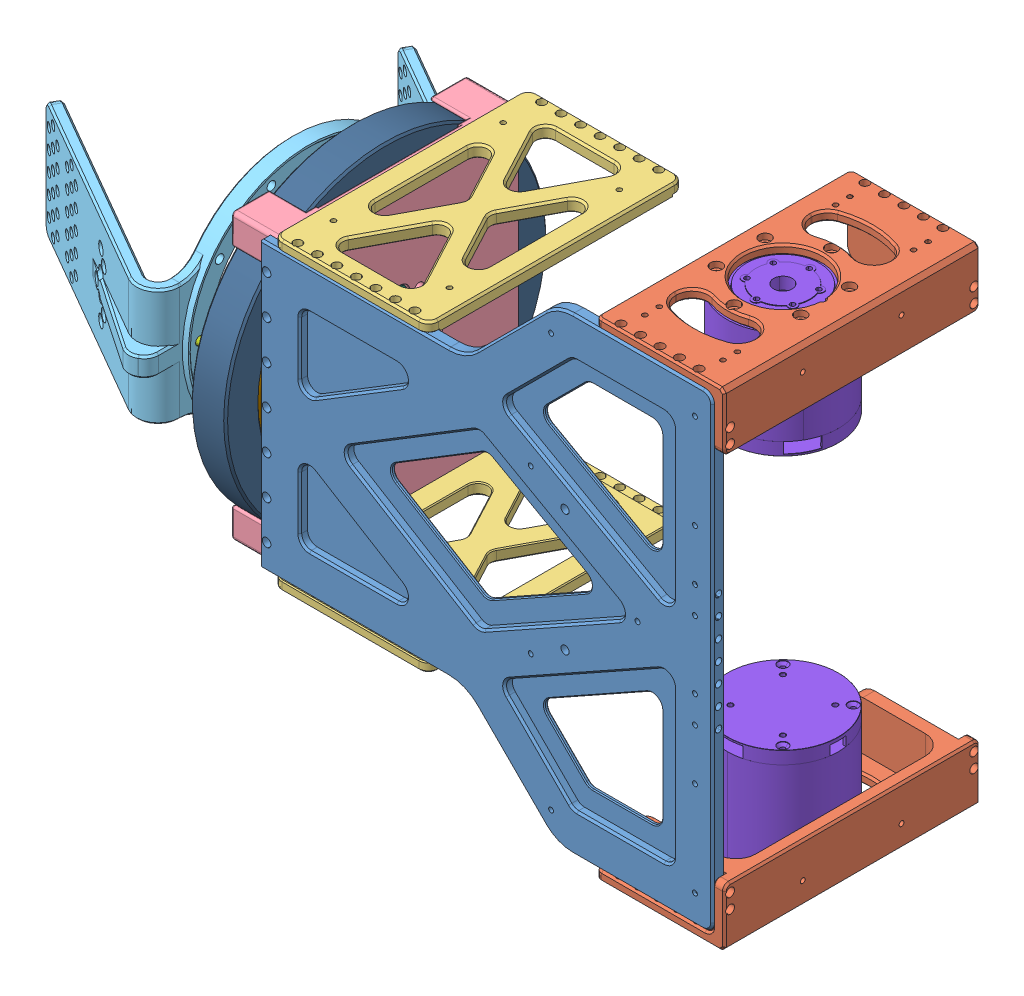
SolidWorks assembly ATOM01胸椎装配体, configuration 默认. Lengths in mm.
Overall size (401.98 250.34 188.64).
24 component instances, 10 part files, 46 mates.
Components (placement in the parent):
- RB000171_01_胸腔前后夹板-1: RB000171_01_胸腔前后夹板 [默认] at (-119.7201 -157.3473 179.5005) size (231.68 240 6)
- RB000160_02_肩膀-1: RB000160_02_肩膀 [默认] at (-119.7201 -37.3473 58.5005) x (-1 0 0) z (0 1 0) size (66 131 30.17)
- RB000160_02_肩膀-2: RB000160_02_肩膀 [默认] at (-119.7201 -277.3473 179.5005) x (-1 0 0) z (0 -1 0) size (66 131 30.17)
- RB000157_01_侧板横板-1: RB000157_01_侧板横板 [默认] at (-119.7201 -84.3473 119.0005) x (0 0 -1) z (0 1 0) size (131 80 6)
- RB000157_01_侧板横板-2: RB000157_01_侧板横板 [默认] at (-119.7201 -230.3473 119.0005) x (0 0 1) z (0 -1 0) size (131 80 6)
- RB000159_02_电池底盖-1: RB000159_02_电池底盖 [默认] at (-119.7201 -157.3473 119.0005) x (0 0 -1) z (1 0 0) size (121 146 26)
- RB000164_01_髋关节固定-1: RB000164_01_髋关节固定 [默认] at (-157.9201 -157.3473 119.0005) x (0 0 1) z (-1 0 0) size (186.22 124 120.18)
- GB╱T 70.1-2008[内六角圆柱头螺钉M5×10]-1: GB╱T 70.1-2008[内六角圆柱头螺钉M5×10] [M5×10] at (-108.7201 -157.3473 101.0005) x (-1 0 0) z (0 -0.924225 -0.381849) size (15 8.5 8.5)
- GB╱T 70.1-2008[内六角圆柱头螺钉M5×10]-2: GB╱T 70.1-2008[内六角圆柱头螺钉M5×10] [M5×10] at (-108.7201 -166.3473 103.412) x (-1 0 0) z (0 -0.924225 -0.381849) size (15 8.5 8.5)
- GB╱T 70.1-2008[内六角圆柱头螺钉M5×10]-3: GB╱T 70.1-2008[内六角圆柱头螺钉M5×10] [M5×10] at (-108.7201 -148.3473 134.5889) x (-1 0 0) z (0 -0.924225 -0.381849) size (15 8.5 8.5)
- GB╱T 70.1-2008[内六角圆柱头螺钉M5×10]-4: GB╱T 70.1-2008[内六角圆柱头螺钉M5×10] [M5×10] at (-108.7201 -141.7589 128.0005) x (-1 0 0) z (0 -0.924225 -0.381849) size (15 8.5 8.5)
- GB╱T 70.1-2008[内六角圆柱头螺钉M5×10]-5: GB╱T 70.1-2008[内六角圆柱头螺钉M5×10] [M5×10] at (-108.7201 -175.3473 119.0005) x (-1 0 0) z (0 -0.924225 -0.381849) size (15 8.5 8.5)
- GB╱T 70.1-2008[内六角圆柱头螺钉M5×10]-6: GB╱T 70.1-2008[内六角圆柱头螺钉M5×10] [M5×10] at (-108.7201 -166.3473 134.5889) x (-1 0 0) z (0 -0.924225 -0.381849) size (15 8.5 8.5)
- GB╱T 70.1-2008[内六角圆柱头螺钉M5×10]-7: GB╱T 70.1-2008[内六角圆柱头螺钉M5×10] [M5×10] at (-108.7201 -172.9358 128.0005) x (-1 0 0) z (0 -0.924225 -0.381849) size (15 8.5 8.5)
- GB╱T 70.1-2008[内六角圆柱头螺钉M5×10]-8: GB╱T 70.1-2008[内六角圆柱头螺钉M5×10] [M5×10] at (-108.7201 -139.3473 119.0005) x (-1 0 0) z (0 -0.924225 -0.381849) size (15 8.5 8.5)
- GB╱T 70.1-2008[内六角圆柱头螺钉M5×10]-9: GB╱T 70.1-2008[内六角圆柱头螺钉M5×10] [M5×10] at (-108.7201 -148.3473 103.412) x (-1 0 0) z (0 -0.924225 -0.381849) size (15 8.5 8.5)
- GB╱T 70.1-2008[内六角圆柱头螺钉M4×12]-1: GB╱T 70.1-2008[内六角圆柱头螺钉M4×12] [默认] at (-167.9201 -157.3473 66.0005) x (1 0 0) z (0 0 -1) size (16 7 7)
- GB╱T 70.1-2008[内六角圆柱头螺钉M4×12]-3: GB╱T 70.1-2008[内六角圆柱头螺钉M4×12] [默认] at (-167.9201 -188.4999 161.8784) x (1 0 0) z (0 0 -1) size (16 7 7)
- GB╱T 70.1-2008[内六角圆柱头螺钉M4×12]-4: GB╱T 70.1-2008[内六角圆柱头螺钉M4×12] [默认] at (-167.9201 -157.3473 172.0005) x (1 0 0) z (0 0 -1) size (16 7 7)
- GB╱T 70.1-2008[内六角圆柱头螺钉M4×12]-6: GB╱T 70.1-2008[内六角圆柱头螺钉M4×12] [默认] at (-167.9201 -126.1947 76.1226) x (1 0 0) z (0 0 -1) size (16 7 7)
- DM 4340 rau 3505 电机 3D-1: DM 4340 rau 3505 电机 3D [默认] at (87.9558 -279.0973 119.0005) size (57 56.5 57)
- DM 4340 rau 3505 电机 3D-2: DM 4340 rau 3505 电机 3D [默认] at (87.9558 -35.5973 119.0005) x (-0.5 0 0.866025) z (0.866025 0 0.5) size (57 56.5 57)
- RB000174_03_腰部支撑-1: RB000174_03_腰部支撑 [默认] at (-133.2201 -157.3473 119.0005) x (0 -0.978148 -0.207912) z (-1 0 0) size (142 142 21)
- 滚动轴承-1: 滚动轴承 [默认] at (-115.2201 -157.3473 119.0005) x (0 1 0) z (0 0 1) size (165 18 165)
Mates (geometry in assembly coordinates):
- 同心5: concentric aligned: cylinder of RB000171_01_胸腔前后夹板-1 through (117.4558 -50.3473 181.5005) axis (1 0 0) radius 1.65; cylinder of RB000160_02_肩膀-1 through (105.4558 -50.3473 181.5005) axis (1 0 0) radius 2.2
- 同心6: concentric aligned: cylinder of RB000171_01_胸腔前后夹板-1 through (107.4558 -37.3473 181.5005) axis (0 1 0) radius 1.65; cylinder of RB000160_02_肩膀-1 through (107.4558 -50.3473 181.5005) axis (0 1 0) radius 2.2
- 同心7: concentric aligned: cylinder of RB000171_01_胸腔前后夹板-1 through (117.4558 -264.3473 181.5005) axis (1 0 0) radius 1.65; cylinder of RB000160_02_肩膀-2 through (105.4558 -264.3473 181.5005) axis (1 0 0) radius 2.2
- 同心8: concentric aligned: cylinder of RB000171_01_胸腔前后夹板-1 through (107.4558 -277.3473 181.5005) axis (0 -1 0) radius 1.65; cylinder of RB000160_02_肩膀-2 through (107.4558 -264.3473 181.5005) axis (0 -1 0) radius 2.2
- 重合1: coincident anti-aligned: plane of RB000171_01_胸腔前后夹板-1 through (-108.2201 -84.3473 178.5005) normal (0 1 0); plane of RB000157_01_侧板横板-1 through (-119.7201 -84.3473 119.0005) normal (0 -1 0)
- 同心9: concentric aligned: cylinder of RB000171_01_胸腔前后夹板-1 through (-38.2201 -84.3473 181.5005) axis (0 1 0) radius 1.65; cylinder of RB000157_01_侧板横板-1 through (-38.2201 -90.3473 181.5005) axis (0 1 0) radius 2.2
- 同心10: concentric aligned: cylinder of RB000171_01_胸腔前后夹板-1 through (-98.2201 -84.3473 181.5005) axis (0 1 0) radius 1.65; cylinder of RB000157_01_侧板横板-1 through (-98.2201 -90.3473 181.5005) axis (0 1 0) radius 2.2
- 重合2: coincident anti-aligned: plane of RB000171_01_胸腔前后夹板-1 through (-108.2201 -230.3473 178.5005) normal (0 -1 0); plane of RB000157_01_侧板横板-2 through (-119.7201 -230.3473 119.0005) normal (0 1 0)
- 同心11: concentric aligned: cylinder of RB000171_01_胸腔前后夹板-1 through (-38.2201 -230.3473 181.5005) axis (0 -1 0) radius 1.65; cylinder of RB000157_01_侧板横板-2 through (-38.2201 -224.3473 181.5005) axis (0 -1 0) radius 2.2
- 同心12: concentric aligned: cylinder of RB000171_01_胸腔前后夹板-1 through (-98.2201 -230.3473 181.5005) axis (0 -1 0) radius 1.65; cylinder of RB000157_01_侧板横板-2 through (-98.2201 -224.3473 181.5005) axis (0 -1 0) radius 2.2
- 重合3: coincident anti-aligned: plane of RB000171_01_胸腔前后夹板-1 through (-119.7201 -157.3473 179.5005) normal (0 0 -1); plane of RB000159_02_电池底盖-1 through (-108.2201 -84.3473 179.5005) normal (0 0 1)
- 同心13: concentric aligned: cylinder of RB000171_01_胸腔前后夹板-1 through (-111.2201 -217.3473 178.5005) axis (0 0 1) radius 2.2; cylinder of RB000159_02_电池底盖-1 through (-111.2201 -217.3473 179.5005) axis (0 0 1) radius 1.65
- 同心14: concentric aligned: cylinder of RB000171_01_胸腔前后夹板-1 through (-111.2201 -97.3473 178.5005) axis (0 0 1) radius 2.2; cylinder of RB000159_02_电池底盖-1 through (-111.2201 -97.3473 179.5005) axis (0 0 1) radius 1.65
- 平行1: parallel anti-aligned: plane of RB000157_01_侧板横板-2 through (-119.7201 -235.3473 119.0005) normal (0 -1 0); plane of RB000164_01_髋关节固定-1 through (-163.9201 -127.3473 64.7418) normal (0 1 0)
- 重合9: coincident aligned: plane of GB╱T 70.1-2008[内六角圆柱头螺钉M5×10]-2 through (-113.7201 -164.7245 99.4841) normal (-1 0 0); plane of GB╱T 70.1-2008[内六角圆柱头螺钉M5×10]-3 through (-113.7201 -146.7245 130.661) normal (-1 0 0)
- 重合10: coincident aligned: plane of GB╱T 70.1-2008[内六角圆柱头螺钉M5×10]-3 through (-113.7201 -146.7245 130.661) normal (-1 0 0); plane of GB╱T 70.1-2008[内六角圆柱头螺钉M5×10]-4 through (-113.7201 -140.136 124.0725) normal (-1 0 0)
- 重合11: coincident aligned: plane of GB╱T 70.1-2008[内六角圆柱头螺钉M5×10]-1 through (-113.7201 -155.7245 97.0725) normal (-1 0 0); plane of GB╱T 70.1-2008[内六角圆柱头螺钉M5×10]-4 through (-113.7201 -140.136 124.0725) normal (-1 0 0)
- 重合12: coincident aligned: plane of GB╱T 70.1-2008[内六角圆柱头螺钉M5×10]-1 through (-113.7201 -155.7245 97.0725) normal (-1 0 0); plane of GB╱T 70.1-2008[内六角圆柱头螺钉M5×10]-9 through (-113.7201 -146.7245 99.4841) normal (-1 0 0)
- 重合13: coincident aligned: plane of GB╱T 70.1-2008[内六角圆柱头螺钉M5×10]-5 through (-113.7201 -173.7245 115.0725) normal (-1 0 0); plane of GB╱T 70.1-2008[内六角圆柱头螺钉M5×10]-9 through (-113.7201 -146.7245 99.4841) normal (-1 0 0)
- 重合14: coincident aligned: plane of GB╱T 70.1-2008[内六角圆柱头螺钉M5×10]-5 through (-113.7201 -173.7245 115.0725) normal (-1 0 0); plane of GB╱T 70.1-2008[内六角圆柱头螺钉M5×10]-6 through (-113.7201 -164.7245 130.661) normal (-1 0 0)
- 重合15: coincident aligned: plane of GB╱T 70.1-2008[内六角圆柱头螺钉M5×10]-6 through (-113.7201 -164.7245 130.661) normal (-1 0 0); plane of GB╱T 70.1-2008[内六角圆柱头螺钉M5×10]-7 through (-113.7201 -171.3129 124.0725) normal (-1 0 0)
- 重合16: coincident aligned: plane of GB╱T 70.1-2008[内六角圆柱头螺钉M5×10]-7 through (-113.7201 -171.3129 124.0725) normal (-1 0 0); plane of GB╱T 70.1-2008[内六角圆柱头螺钉M5×10]-8 through (-113.7201 -137.7245 115.0725) normal (-1 0 0)
- 重合17: coincident anti-aligned: plane of RB000159_02_电池底盖-1 through (-113.7201 -166.3473 131.6889) normal (1 0 0); plane of GB╱T 70.1-2008[内六角圆柱头螺钉M5×10]-8 through (-113.7201 -137.7245 115.0725) normal (-1 0 0)
- 同心23: concentric anti-aligned: cylinder of RB000159_02_电池底盖-1 through (-108.2201 -166.3473 134.5889) axis (1 0 0) radius 2.9; cylinder of GB╱T 70.1-2008[内六角圆柱头螺钉M5×10]-6 through (-108.7201 -166.3473 134.5889) axis (-1 0 0) radius 4.25
- 同心24: concentric anti-aligned: cylinder of RB000159_02_电池底盖-1 through (-108.2201 -172.9358 128.0005) axis (1 0 0) radius 2.9; cylinder of GB╱T 70.1-2008[内六角圆柱头螺钉M5×10]-7 through (-108.7201 -172.9358 128.0005) axis (-1 0 0) radius 4.25
- 同心25: concentric anti-aligned: cylinder of RB000159_02_电池底盖-1 through (-108.2201 -175.3473 119.0005) axis (1 0 0) radius 2.9; cylinder of GB╱T 70.1-2008[内六角圆柱头螺钉M5×10]-5 through (-108.7201 -175.3473 119.0005) axis (-1 0 0) radius 4.25
- 同心26: concentric anti-aligned: cylinder of GB╱T 70.1-2008[内六角圆柱头螺钉M5×10]-2 through (-108.7201 -166.3473 103.412) axis (-1 0 0) radius 4.25; cylinder of RB000159_02_电池底盖-1 through (-108.2201 -166.3473 103.412) axis (1 0 0) radius 2.9
- 同心27: concentric anti-aligned: cylinder of RB000159_02_电池底盖-1 through (-108.2201 -157.3473 101.0005) axis (1 0 0) radius 2.9; cylinder of GB╱T 70.1-2008[内六角圆柱头螺钉M5×10]-1 through (-108.7201 -157.3473 101.0005) axis (-1 0 0) radius 4.25
- 同心28: concentric anti-aligned: cylinder of RB000159_02_电池底盖-1 through (-108.2201 -148.3473 103.412) axis (1 0 0) radius 2.9; cylinder of GB╱T 70.1-2008[内六角圆柱头螺钉M5×10]-9 through (-108.7201 -148.3473 103.412) axis (-1 0 0) radius 4.25
- 同心29: concentric anti-aligned: cylinder of RB000159_02_电池底盖-1 through (-108.2201 -141.7589 128.0005) axis (1 0 0) radius 2.9; cylinder of GB╱T 70.1-2008[内六角圆柱头螺钉M5×10]-4 through (-108.7201 -141.7589 128.0005) axis (-1 0 0) radius 4.25
- 同心30: concentric anti-aligned: cylinder of RB000159_02_电池底盖-1 through (-108.2201 -148.3473 134.5889) axis (1 0 0) radius 2.9; cylinder of GB╱T 70.1-2008[内六角圆柱头螺钉M5×10]-3 through (-108.7201 -148.3473 134.5889) axis (-1 0 0) radius 4.25
- 重合20: coincident aligned: plane of GB╱T 70.1-2008[内六角圆柱头螺钉M4×12]-3 through (-163.9201 -191.9999 161.8784) normal (1 0 0); plane of GB╱T 70.1-2008[内六角圆柱头螺钉M4×12]-4 through (-163.9201 -160.8473 172.0005) normal (1 0 0)
- 重合27: coincident anti-aligned: plane of RB000164_01_髋关节固定-1 through (-163.9201 -157.3473 119.0005) normal (-1 0 0); plane of GB╱T 70.1-2008[内六角圆柱头螺钉M4×12]-1 through (-163.9201 -160.8473 66.0005) normal (1 0 0)
- 同心32: concentric aligned: cylinder of RB000164_01_髋关节固定-1 through (-165.9201 -157.3473 66.0005) axis (1 0 0) radius 2.2; cylinder of GB╱T 70.1-2008[内六角圆柱头螺钉M4×12]-1 through (-167.9201 -157.3473 66.0005) axis (1 0 0) radius 3.5
- 同心33: concentric aligned: cylinder of RB000164_01_髋关节固定-1 through (-165.9201 -126.1947 76.1226) axis (1 0 0) radius 2.2; cylinder of GB╱T 70.1-2008[内六角圆柱头螺钉M4×12]-6 through (-167.9201 -126.1947 76.1226) axis (1 0 0) radius 3.5
- 同心37: concentric aligned: cylinder of RB000164_01_髋关节固定-1 through (-165.9201 -157.3473 172.0005) axis (1 0 0) radius 2.2; cylinder of GB╱T 70.1-2008[内六角圆柱头螺钉M4×12]-4 through (-167.9201 -157.3473 172.0005) axis (1 0 0) radius 3.5
- 同心38: concentric aligned: cylinder of RB000164_01_髋关节固定-1 through (-165.9201 -188.4999 161.8784) axis (1 0 0) radius 2.2; cylinder of GB╱T 70.1-2008[内六角圆柱头螺钉M4×12]-3 through (-167.9201 -188.4999 161.8784) axis (1 0 0) radius 3.5
- 重合28: coincident anti-aligned: plane of RB000160_02_肩膀-2 through (-119.7201 -277.3473 179.5005) normal (0 1 0); plane of DM 4340 rau 3505 电机 3D-1 through (106.9558 -277.3473 119.0005) normal (0 -1 0)
- 同心42: concentric aligned: cylinder of RB000160_02_肩膀-2 through (87.9558 -272.3473 119.0005) axis (0 -1 0) radius 20; cylinder of DM 4340 rau 3505 电机 3D-1 through (87.9558 -279.0973 119.0005) axis (0 -1 0) radius 28.5
- 同心43: concentric aligned: cylinder of RB000160_02_肩膀-2 through (109.6064 -279.3473 131.5005) axis (0 -1 0) radius 3; cylinder of DM 4340 rau 3505 电机 3D-1 through (109.6064 -277.3473 131.5005) axis (0 -1 0) radius 1.25
- 同心44: concentric aligned: cylinder of RB000160_02_肩膀-1 through (87.9558 -42.3473 119.0005) axis (0 1 0) radius 20; cylinder of DM 4340 rau 3505 电机 3D-2 through (87.9558 -35.5973 119.0005) axis (0 1 0) radius 28.5
- 重合29: coincident anti-aligned: plane of RB000160_02_肩膀-1 through (-119.7201 -37.3473 58.5005) normal (0 -1 0); plane of DM 4340 rau 3505 电机 3D-2 through (78.4558 -37.3473 135.4549) normal (0 1 0)
- 同心45: concentric aligned: cylinder of RB000160_02_肩膀-1 through (109.6064 -35.3473 106.5005) axis (0 1 0) radius 3; cylinder of DM 4340 rau 3505 电机 3D-2 through (109.6064 -37.3473 106.5005) axis (0 1 0) radius 1.25
- 同心46: concentric anti-aligned: cylinder of RB000164_01_髋关节固定-1 through (-163.9201 -157.3473 119.0005) axis (1 0 0) radius 62; cylinder of RB000174_03_腰部支撑-1 through (-115.2201 -157.3473 119.0005) axis (-1 0 0) radius 49
- 同心48: concentric anti-aligned: cylinder of RB000174_03_腰部支撑-1 through (69.6277 -157.3473 119.0005) axis (-1 0 0) radius 65; cylinder of 滚动轴承-1 through (-133.2201 -157.3473 119.0005) axis (1 0 0) radius 65
- 重合31: coincident anti-aligned: plane of RB000174_03_腰部支撑-1 through (-133.2201 -157.3473 119.0005) normal (1 0 0); plane of 滚动轴承-1 through (-133.2201 -157.3473 119.0005) normal (-1 0 0)
